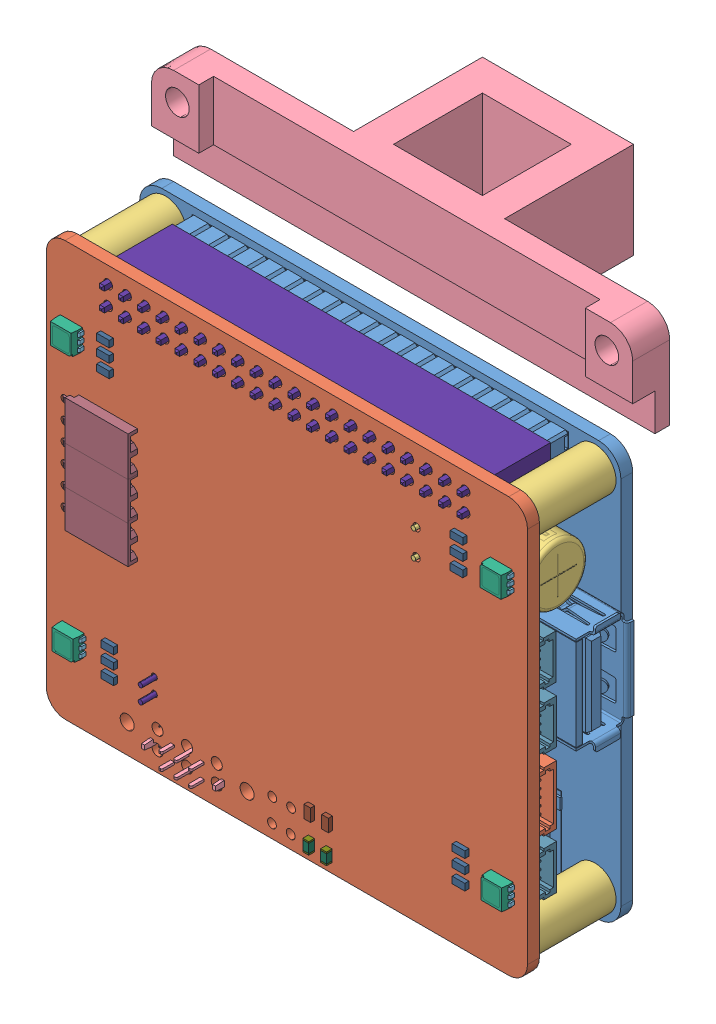
SolidWorks assembly STMf303 hat + RPi 3A+, configuration Default. Lengths in mm.
Overall size (68.17 71.5 38.51).
304 component instances, 41 part files, 9 mates.
Components (placement in the parent):
- Raspberry PI 3 Model A+-1: Raspberry PI 3 Model A+ [Défaut] at (135.3946 10.6154 11.2635) size (68.17 58.5 11.94)
- FC_PiHat_REV1-1: FC_PiHat_REV1 [Default] at (41.2941 -16.4646 23.8635) x (-1 0 0) z (0 0 -1) size (65 56 12.01)
  - FC_PiHat_REV1.step-1: FC_PiHat_REV1.step [Default] at origin size (65 56 12.01)
    - J7FC_PiHat_REV1.step-1: J7FC_PiHat_REV1.step [Default] at origin size (8 4.95 2.96)
      - SM06B-SRSS-TB.step-1: SM06B-SRSS-TB.step [Default] at (13.3 4.6 -0.3) x (1 0 0) z (0 -1 0) size (8 2.96 4.95)
    - C10FC_PiHat_REV1.step-1: C10FC_PiHat_REV1.step [Default] at origin size (13.96 8.06 10.04)
      - User_Library-Cap_electro_8x11_5x3_5mm_RA.step-1: User_Library-Cap_electro_8x11_5x3_5mm_RA.step [Default] at (13.5254 44.5 4) x (0 1 0) z (0 0 1) size (8.06 13.96 10.04)
    - J11FC_PiHat_REV1.step-1: J11FC_PiHat_REV1.step [Default] at origin size (10 6 9.8)
      - User_Library-EG1940-ND.step-1: User_Library-EG1940-ND.step [Default] at (40.9499 0.2249 0) x (1 0 0) z (0 0 1) size (10 6 9.8)
    - D4FC_PiHat_REV1.step-1: D4FC_PiHat_REV1.step [Default] at origin size (3.4 2.8 1.85)
      - User_Library-RGB_LED_Zwart_ASMT-YTC2-0AA02.step-1: User_Library-RGB_LED_Zwart_ASMT-YTC2-0AA02.step [Default] at (2.2908 8.9737 -1.6023) x (-1 0 0) z (0 -1 0) size (3.4 1.85 2.8)
        - Pootje_RGB_LED.step-1: Pootje_RGB_LED.step [Default] at (-0.3594 -0.1975 0.3238) size (0.9 1.1 0.5)
        - ASMT-YTC2-0AA02.step-1: ASMT-YTC2-0AA02.step [Default] at (-2.6594 -0.3475 0.5738) size (3 1.8 2.8)
        - Pootje_RGB_LED.step-2: Pootje_RGB_LED.step [Default] at (-0.3594 -0.1975 -0.5762) size (0.9 1.1 0.5)
        - Pootje_RGB_LED.step-3: Pootje_RGB_LED.step [Default] at (-0.3594 -0.1975 -1.4762) size (0.9 1.1 0.5)
        - Pootje_RGB_LED.step-4: Pootje_RGB_LED.step [Default] at (-1.9594 -0.1975 -1.9762) x (-1 0 0) z (0 0 -1) size (0.9 1.1 0.5)
        - Pootje_RGB_LED.step-5: Pootje_RGB_LED.step [Default] at (-1.9594 -0.1975 -1.0762) x (-1 0 0) z (0 0 -1) size (0.9 1.1 0.5)
        - Pootje_RGB_LED.step-6: Pootje_RGB_LED.step [Default] at (-1.9594 -0.1975 -0.1762) x (-1 0 0) z (0 0 -1) size (0.9 1.1 0.5)
    - D3FC_PiHat_REV1.step-1: D3FC_PiHat_REV1.step [Default] at origin size (3.4 2.8 1.85)
      - User_Library-RGB_LED_Zwart_ASMT-YTC2-0AA02.step-1: User_Library-RGB_LED_Zwart_ASMT-YTC2-0AA02.step [Default] at (2.3908 45.4737 -1.6023) x (-1 0 0) z (0 -1 0) size (3.4 1.85 2.8)
        - Pootje_RGB_LED.step-1: Pootje_RGB_LED.step [Default] at (-0.3594 -0.1975 0.3238) size (0.9 1.1 0.5)
        - ASMT-YTC2-0AA02.step-1: ASMT-YTC2-0AA02.step [Default] at (-2.6594 -0.3475 0.5738) size (3 1.8 2.8)
        - Pootje_RGB_LED.step-2: Pootje_RGB_LED.step [Default] at (-0.3594 -0.1975 -0.5762) size (0.9 1.1 0.5)
        - Pootje_RGB_LED.step-3: Pootje_RGB_LED.step [Default] at (-0.3594 -0.1975 -1.4762) size (0.9 1.1 0.5)
        - Pootje_RGB_LED.step-4: Pootje_RGB_LED.step [Default] at (-1.9594 -0.1975 -1.9762) x (-1 0 0) z (0 0 -1) size (0.9 1.1 0.5)
        - Pootje_RGB_LED.step-5: Pootje_RGB_LED.step [Default] at (-1.9594 -0.1975 -1.0762) x (-1 0 0) z (0 0 -1) size (0.9 1.1 0.5)
        - Pootje_RGB_LED.step-6: Pootje_RGB_LED.step [Default] at (-1.9594 -0.1975 -0.1762) x (-1 0 0) z (0 0 -1) size (0.9 1.1 0.5)
    - D2FC_PiHat_REV1.step-1: D2FC_PiHat_REV1.step [Default] at origin size (3.4 2.8 1.85)
      - User_Library-RGB_LED_Zwart_ASMT-YTC2-0AA02.step-1: User_Library-RGB_LED_Zwart_ASMT-YTC2-0AA02.step [Default] at (62.5092 10.7763 -1.6023) x (1 0 0) z (0 1 0) size (3.4 1.85 2.8)
        - Pootje_RGB_LED.step-1: Pootje_RGB_LED.step [Default] at (-0.3594 -0.1975 0.3238) size (0.9 1.1 0.5)
        - ASMT-YTC2-0AA02.step-1: ASMT-YTC2-0AA02.step [Default] at (-2.6594 -0.3475 0.5738) size (3 1.8 2.8)
        - Pootje_RGB_LED.step-2: Pootje_RGB_LED.step [Default] at (-0.3594 -0.1975 -0.5762) size (0.9 1.1 0.5)
        - Pootje_RGB_LED.step-3: Pootje_RGB_LED.step [Default] at (-0.3594 -0.1975 -1.4762) size (0.9 1.1 0.5)
        - Pootje_RGB_LED.step-4: Pootje_RGB_LED.step [Default] at (-1.9594 -0.1975 -1.9762) x (-1 0 0) z (0 0 -1) size (0.9 1.1 0.5)
        - Pootje_RGB_LED.step-5: Pootje_RGB_LED.step [Default] at (-1.9594 -0.1975 -1.0762) x (-1 0 0) z (0 0 -1) size (0.9 1.1 0.5)
        - Pootje_RGB_LED.step-6: Pootje_RGB_LED.step [Default] at (-1.9594 -0.1975 -0.1762) x (-1 0 0) z (0 0 -1) size (0.9 1.1 0.5)
    - D1FC_PiHat_REV1.step-1: D1FC_PiHat_REV1.step [Default] at origin size (3.4 2.8 1.85)
      - User_Library-RGB_LED_Zwart_ASMT-YTC2-0AA02.step-1: User_Library-RGB_LED_Zwart_ASMT-YTC2-0AA02.step [Default] at (62.7592 46.4263 -1.6023) x (1 0 0) z (0 1 0) size (3.4 1.85 2.8)
        - Pootje_RGB_LED.step-1: Pootje_RGB_LED.step [Default] at (-0.3594 -0.1975 0.3238) size (0.9 1.1 0.5)
        - ASMT-YTC2-0AA02.step-1: ASMT-YTC2-0AA02.step [Default] at (-2.6594 -0.3475 0.5738) size (3 1.8 2.8)
        - Pootje_RGB_LED.step-2: Pootje_RGB_LED.step [Default] at (-0.3594 -0.1975 -0.5762) size (0.9 1.1 0.5)
        - Pootje_RGB_LED.step-3: Pootje_RGB_LED.step [Default] at (-0.3594 -0.1975 -1.4762) size (0.9 1.1 0.5)
        - Pootje_RGB_LED.step-4: Pootje_RGB_LED.step [Default] at (-1.9594 -0.1975 -1.9762) x (-1 0 0) z (0 0 -1) size (0.9 1.1 0.5)
        - Pootje_RGB_LED.step-5: Pootje_RGB_LED.step [Default] at (-1.9594 -0.1975 -1.0762) x (-1 0 0) z (0 0 -1) size (0.9 1.1 0.5)
        - Pootje_RGB_LED.step-6: Pootje_RGB_LED.step [Default] at (-1.9594 -0.1975 -0.1762) x (-1 0 0) z (0 0 -1) size (0.9 1.1 0.5)
    - S1FC_PiHat_REV1.step-1: S1FC_PiHat_REV1.step [Default] at origin size (4.1 4.1 0.81)
      - 5843174976.step-1: 5843174976.step [Default] at (40.7 32.3 0) size (4.1 4.1 0.81)
        - Body.step-1: Body.step [Default] at (-2.05 -2.05 0)
          - Open_CASCADE_STEP_translator_6.8_14.2.1.x_t-1: Open_CASCADE_STEP_translator_6.8_14.2.1.x_t [Default] at origin
        - Open_CASCADE_STEP_translator_6.8_14.1.step-1: Open_CASCADE_STEP_translator_6.8_14.1.step [Default] at (-2.05 -2.05 0) size (0.52 0.52 0.01)
        - Thermal_Shape.step-1: Thermal_Shape.step [Default] at (-1.3 -1.35 -0.001) size (2.6 2.7 0)
        - Pin_Shape.step-1: Pin_Shape.step [Default] at (-2.05 -1.37 0) size (0.35 0.24 0)
        - Pin_Shape.step-2: Pin_Shape.step [Default] at (2.05 1.37 0) x (-1 0 0) z (0 0 1) size (0.35 0.24 0)
        - Pin_Shape.step-3: Pin_Shape.step [Default] at (-2.05 -0.87 0) size (0.35 0.24 0)
        - Pin_Shape.step-4: Pin_Shape.step [Default] at (2.05 0.87 0) x (-1 0 0) z (0 0 1) size (0.35 0.24 0)
        - Pin_Shape.step-5: Pin_Shape.step [Default] at (-2.05 -0.37 0) size (0.35 0.24 0)
        - Pin_Shape.step-6: Pin_Shape.step [Default] at (2.05 0.37 0) x (-1 0 0) z (0 0 1) size (0.35 0.24 0)
        - Pin_Shape.step-7: Pin_Shape.step [Default] at (-2.05 0.13 0) size (0.35 0.24 0)
        - Pin_Shape.step-8: Pin_Shape.step [Default] at (2.05 -0.13 0) x (-1 0 0) z (0 0 1) size (0.35 0.24 0)
        - Pin_Shape.step-9: Pin_Shape.step [Default] at (-2.05 0.63 0) size (0.35 0.24 0)
        - Pin_Shape.step-10: Pin_Shape.step [Default] at (2.05 -0.63 0) x (-1 0 0) z (0 0 1) size (0.35 0.24 0)
        - Pin_Shape.step-11: Pin_Shape.step [Default] at (-2.05 1.13 0) size (0.35 0.24 0)
        - Pin_Shape.step-12: Pin_Shape.step [Default] at (2.05 -1.13 0) x (-1 0 0) z (0 0 1) size (0.35 0.24 0)
        - Pin_Shape.step-13: Pin_Shape.step [Default] at (-1.13 -2.05 0) x (0 1 0) z (0 0 1) size (0.35 0.24 0)
        - Pin_Shape.step-14: Pin_Shape.step [Default] at (1.13 2.05 0) x (0 -1 0) z (0 0 1) size (0.35 0.24 0)
        - Pin_Shape.step-15: Pin_Shape.step [Default] at (-0.63 -2.05 0) x (0 1 0) z (0 0 1) size (0.35 0.24 0)
        - Pin_Shape.step-16: Pin_Shape.step [Default] at (0.63 2.05 0) x (0 -1 0) z (0 0 1) size (0.35 0.24 0)
        - Pin_Shape.step-17: Pin_Shape.step [Default] at (-0.13 -2.05 0) x (0 1 0) z (0 0 1) size (0.35 0.24 0)
        - Pin_Shape.step-18: Pin_Shape.step [Default] at (0.13 2.05 0) x (0 -1 0) z (0 0 1) size (0.35 0.24 0)
        - Pin_Shape.step-19: Pin_Shape.step [Default] at (0.37 -2.05 0) x (0 1 0) z (0 0 1) size (0.35 0.24 0)
        - Pin_Shape.step-20: Pin_Shape.step [Default] at (-0.37 2.05 0) x (0 -1 0) z (0 0 1) size (0.35 0.24 0)
        - Pin_Shape.step-21: Pin_Shape.step [Default] at (0.87 -2.05 0) x (0 1 0) z (0 0 1) size (0.35 0.24 0)
        - Pin_Shape.step-22: Pin_Shape.step [Default] at (-0.87 2.05 0) x (0 -1 0) z (0 0 1) size (0.35 0.24 0)
        - Pin_Shape.step-23: Pin_Shape.step [Default] at (1.37 -2.05 0) x (0 1 0) z (0 0 1) size (0.35 0.24 0)
        - Pin_Shape.step-24: Pin_Shape.step [Default] at (-1.37 2.05 0) x (0 -1 0) z (0 0 1) size (0.35 0.24 0)
    - R14FC_PiHat_REV1.step-1: R14FC_PiHat_REV1.step [Default] at origin size (1.7 0.9 0.55)
      - 6063442624.step-1: 6063442624.step [Default] at (8.7742 7.9 -2.1523) size (1.7 0.9 0.55)
        - Extruded.step-1: Extruded.step [Default] at origin size (1.7 0.9 0.55)
    - R13FC_PiHat_REV1.step-1: R13FC_PiHat_REV1.step [Default] at origin size (1.7 0.9 0.55)
      - 6063442624.step-1: 6063442624.step [Default] at (8.7742 9.8048 -2.1523) size (1.7 0.9 0.55)
        - Extruded.step-1: Extruded.step [Default] at origin size (1.7 0.9 0.55)
    - R12FC_PiHat_REV1.step-1: R12FC_PiHat_REV1.step [Default] at origin size (1.7 0.9 0.55)
      - 6063442624.step-1: 6063442624.step [Default] at (8.7742 11.7 -2.1523) size (1.7 0.9 0.55)
        - Extruded.step-1: Extruded.step [Default] at origin size (1.7 0.9 0.55)
    - R11FC_PiHat_REV1.step-1: R11FC_PiHat_REV1.step [Default] at origin size (1.7 0.9 0.55)
      - 6063442624.step-1: 6063442624.step [Default] at (9.05 44.4 -2.1523) size (1.7 0.9 0.55)
        - Extruded.step-1: Extruded.step [Default] at origin size (1.7 0.9 0.55)
    - R10FC_PiHat_REV1.step-1: R10FC_PiHat_REV1.step [Default] at origin size (1.7 0.9 0.55)
      - 6063442624.step-1: 6063442624.step [Default] at (9.05 46.3 -2.1523) size (1.7 0.9 0.55)
        - Extruded.step-1: Extruded.step [Default] at origin size (1.7 0.9 0.55)
    - R9FC_PiHat_REV1.step-1: R9FC_PiHat_REV1.step [Default] at origin size (0.9 1.7 0.55)
      - 6063442432.step-1: 6063442432.step [Default] at (59.9 29.7 0) size (0.9 1.7 0.55)
        - Extruded-0.step-1: Extruded-0.step [Default] at origin size (0.9 1.7 0.55)
    - R8FC_PiHat_REV1.step-1: R8FC_PiHat_REV1.step [Default] at origin size (1.7 0.9 0.55)
      - 6063442624.step-1: 6063442624.step [Default] at (9.05 48.2 -2.1523) size (1.7 0.9 0.55)
        - Extruded.step-1: Extruded.step [Default] at origin size (1.7 0.9 0.55)
    - R7FC_PiHat_REV1.step-1: R7FC_PiHat_REV1.step [Default] at origin size (1.84 1.84 0.55)
      - 6063441088.step-1: 6063441088.step [Default] at (39.9 37.9 0) size (1.84 1.84 0.55)
        - Extruded-1.step-1: Extruded-1.step [Default] at origin size (1.84 1.84 0.55)
    - R6FC_PiHat_REV1.step-1: R6FC_PiHat_REV1.step [Default] at origin size (1.7 0.9 0.55)
      - 6063442624.step-1: 6063442624.step [Default] at (56.2 11.8 -2.1523) size (1.7 0.9 0.55)
        - Extruded.step-1: Extruded.step [Default] at origin size (1.7 0.9 0.55)
    - R5FC_PiHat_REV1.step-1: R5FC_PiHat_REV1.step [Default] at origin size (1.7 0.9 0.55)
      - 6063442624.step-1: 6063442624.step [Default] at (56.2 10 -2.1523) size (1.7 0.9 0.55)
        - Extruded.step-1: Extruded.step [Default] at origin size (1.7 0.9 0.55)
    - R4FC_PiHat_REV1.step-1: R4FC_PiHat_REV1.step [Default] at origin size (1.7 0.9 0.55)
      - 6063442624.step-1: 6063442624.step [Default] at (56.2 8.2 -2.1523) size (1.7 0.9 0.55)
        - Extruded.step-1: Extruded.step [Default] at origin size (1.7 0.9 0.55)
    - R3FC_PiHat_REV1.step-1: R3FC_PiHat_REV1.step [Default] at origin size (1.7 0.9 0.55)
      - 6063442624.step-1: 6063442624.step [Default] at (56.8 47.4 -2.1523) size (1.7 0.9 0.55)
        - Extruded.step-1: Extruded.step [Default] at origin size (1.7 0.9 0.55)
    - R2FC_PiHat_REV1.step-1: R2FC_PiHat_REV1.step [Default] at origin size (1.7 0.9 0.55)
      - 6063442624.step-1: 6063442624.step [Default] at (56.8 45.6 -2.1523) size (1.7 0.9 0.55)
        - Extruded.step-1: Extruded.step [Default] at origin size (1.7 0.9 0.55)
    - R1FC_PiHat_REV1.step-1: R1FC_PiHat_REV1.step [Default] at origin size (1.7 0.9 0.55)
      - 6063442624.step-1: 6063442624.step [Default] at (56.8 43.8 -2.1523) size (1.7 0.9 0.55)
        - Extruded.step-1: Extruded.step [Default] at origin size (1.7 0.9 0.55)
    - J8FC_PiHat_REV1.step-1: J8FC_PiHat_REV1.step [Default] at origin size (4.95 8 2.96)
      - SM06B-SRSS-TB.step-1: SM06B-SRSS-TB.step [Default] at (4.55 19.8 -0.3) x (0 -1 0) z (-1 0 0) size (8 2.96 4.95)
    - J6FC_PiHat_REV1.step-1: J6FC_PiHat_REV1.step [Default] at origin size (10.06 15.53 5.7)
      - female_header_a-bl254-ea-g02d.step-1: female_header_a-bl254-ea-g02d.step [Default] at (61.2001 31.0851 -1.6023) x (0 -1 0) z (0 0 -1) size (5.33 10.06 5.7)
      - female_header_a-bl254-ea-g02d.step-2: female_header_a-bl254-ea-g02d.step [Default] at (61.2001 26.0099 -1.6023) x (0 -1 0) z (0 0 -1) size (5.33 10.06 5.7)
      - female_header_a-bl254-ea-g02d.step-3: female_header_a-bl254-ea-g02d.step [Default] at (61.2001 36.2099 -1.6023) x (0 -1 0) z (0 0 -1) size (5.33 10.06 5.7)
    - J4FC_PiHat_REV1.step-1: J4FC_PiHat_REV1.step [Default] at origin size (4.95 6 2.96)
      - SM04B-SRSS-TB.step-1: SM04B-SRSS-TB.step [Default] at (4.55 28.375 -0.3) x (0 -1 0) z (-1 0 0) size (6 2.96 4.95)
    - J3FC_PiHat_REV1.step-1: J3FC_PiHat_REV1.step [Default] at origin size (4.95 6 2.96)
      - SM04B-SRSS-TB.step-1: SM04B-SRSS-TB.step [Default] at (4.55 11.35 -0.3) x (0 -1 0) z (-1 0 0) size (6 2.96 4.95)
    - J2FC_PiHat_REV1.step-1: J2FC_PiHat_REV1.step [Default] at origin size (8 4.95 2.96)
      - SM06B-SRSS-TB.step-1: SM06B-SRSS-TB.step [Default] at (22.8093 4.575 -0.3) x (1 0 0) z (0 -1 0) size (8 2.96 4.95)
    - J1FC_PiHat_REV1.step-1: J1FC_PiHat_REV1.step [Default] at origin size (4.95 6 2.96)
      - SM04B-SRSS-TB.step-1: SM04B-SRSS-TB.step [Default] at (4.625 35.925 -0.3) x (0 -1 0) z (-1 0 0) size (6 2.96 4.95)
    - C4FC_PiHat_REV1.step-1: C4FC_PiHat_REV1.step [Default] at origin size (0.9 1.8 0.9)
      - 6063440896.step-1: 6063440896.step [Default] at (41.3 27.825 0) size (0.9 1.8 0.9)
        - Extruded-2.step-1: Extruded-2.step [Default] at origin size (0.9 1.8 0.9)
    - C3FC_PiHat_REV1.step-1: C3FC_PiHat_REV1.step [Default] at origin size (0.9 1.8 0.9)
      - 6063440896.step-1: 6063440896.step [Default] at (44.1 32.225 0) size (0.9 1.8 0.9)
        - Extruded-2.step-1: Extruded-2.step [Default] at origin size (0.9 1.8 0.9)
    - C2FC_PiHat_REV1.step-1: C2FC_PiHat_REV1.step [Default] at origin size (1.8 0.9 0.9)
      - 6063441280.step-1: 6063441280.step [Default] at (38.125 28.8 0) size (1.8 0.9 0.9)
        - Extruded-3.step-1: Extruded-3.step [Default] at origin size (1.8 0.9 0.9)
    - C1FC_PiHat_REV1.step-1: C1FC_PiHat_REV1.step [Default] at origin size (1.8 0.9 0.9)
      - 6063441280.step-1: 6063441280.step [Default] at (38.125 26.7 0) size (1.8 0.9 0.9)
        - Extruded-3.step-1: Extruded-3.step [Default] at origin size (1.8 0.9 0.9)
    - J5FC_PiHat_REV1.step-1: J5FC_PiHat_REV1.step [Default] at origin size (51.1 5 11.1)
      - User_Library-Header_2x20_2_54mm.step-1: User_Library-Header_2x20_2_54mm.step [Default] at (56.6601 52.5601 0) x (1 0 0) z (0 -1 0) size (51.1 11.1 5)
    - L2FC_PiHat_REV1.step-1: L2FC_PiHat_REV1.step [Default] at origin size (12.5 12.7 6.1)
      - 5843174592.step-1: 5843174592.step [Default] at (40.7 17.6 0) x (0 1 0) z (0 0 1) size (12.7 12.5 6.1)
        - pin.step-1: pin.step [Default] at (6.35 2.8 0) x (-1 0 0) z (0 0 1) size (4.5 5.6 3)
          - Open_CASCADE_STEP_translator_6.8_3.3.1.step-1: Open_CASCADE_STEP_translator_6.8_3.3.1.step [Default] at origin size (4.5 5.6 3)
        - pin.step-2: pin.step [Default] at (-6.35 -2.8 0) size (4.5 5.6 3)
          - Open_CASCADE_STEP_translator_6.8_3.3.1.step-1: Open_CASCADE_STEP_translator_6.8_3.3.1.step [Default] at origin size (4.5 5.6 3)
        - Body.step-1: Body.step [Default] at (0 0 0.1)
          - Open_CASCADE_STEP_translator_6.8_14.2.1.x_t-1: Open_CASCADE_STEP_translator_6.8_14.2.1.x_t [Default] at origin
        - cylinder.step-1: cylinder.step [Default] at (0 0 0.1) size (12.5 12.5 3)
    - U3FC_PiHat_REV1.step-1: U3FC_PiHat_REV1.step [Default] at origin size (10.3 15.24 4.47)
      - 5843175168.step-1: 5843175168.step [Default] at (52.775 32.425 0) x (0 1 0) z (0 0 1) size (15.24 10.3 4.47)
        - Body-1.step-1: Body-1.step [Default] at (-4.575 -5.15 0) size (9.15 10.3 4.47)
          - Open_CASCADE_STEP_translator_6.8_42.2.1.step-1: Open_CASCADE_STEP_translator_6.8_42.2.1.step [Default] at origin size (9.15 10.3 4.47)
        - tab.step-1: tab.step [Default] at (-4.575 -5.15 0) size (9 10.25 0.35)
          - Open_CASCADE_STEP_translator_6.8_42.8.1.step-1: Open_CASCADE_STEP_translator_6.8_42.8.1.step [Default] at origin size (9 10.25 0.35)
        - Open_CASCADE_STEP_translator_6.8_42.1.step-1: Open_CASCADE_STEP_translator_6.8_42.1.step [Default] at (-4.575 -5.15 0) size (1.3 1.3 0.01)
        - Lead.step-1: Lead.step [Default] at (-4.575 -3.4 0) x (-1 0 0) z (0 0 1) size (5.46 0.75 2.33)
        - Lead.step-2: Lead.step [Default] at (-4.575 -1.7 0) x (-1 0 0) z (0 0 1) size (5.46 0.75 2.33)
        - Lead.step-3: Lead.step [Default] at (-4.575 0 0) x (-1 0 0) z (0 0 1) size (5.46 0.75 2.33)
        - Lead.step-4: Lead.step [Default] at (-4.575 1.7 0) x (-1 0 0) z (0 0 1) size (5.46 0.75 2.33)
        - Lead.step-5: Lead.step [Default] at (-4.575 3.4 0) x (-1 0 0) z (0 0 1) size (5.46 0.75 2.33)
      - 5843175168-4.step-1: 5843175168-4.step [Default] at (52.775 32.425 0) x (0 1 0) z (0 0 1) size (2.73 0.75 0.2)
    - D6FC_PiHat_REV1.step-1: D6FC_PiHat_REV1.step [Default] at origin size (7.55 6.23 2.62)
      - 5843175552.step-1: 5843175552.step [Default] at (51.8001 16.8001 0) x (1 0 0) z (0 0 1) size (7.55 6.22 2.62)
        - Body-2.step-1: Body-2.step [Default] at (-3.555 -3.11 0.25) size (7.12 6.22 2.47)
          - Open_CASCADE_STEP_translator_6.8_45.1.1.step-1: Open_CASCADE_STEP_translator_6.8_45.1.1.step [Default] at origin size (7.12 6.22 2.47)
        - Lead-5.step-1: Lead-5.step [Default] at (2.635 0 0) size (1.14 3 1.53)
        - Lead-5.step-2: Lead-5.step [Default] at (-2.635 0 0) x (-1 0 0) z (0 0 1) size (1.14 3 1.53)
    - U2FC_PiHat_REV1.step-1: U2FC_PiHat_REV1.step [Default] at origin size (3.98 3.97 1)
      - 5843176128.step-1: 5843176128.step [Default] at (49.3313 45.4354 0) x (0.707107 -0.707107 0) z (0 0 1) size (2.8 2.91 1)
        - Body-3.step-1: Body-3.step [Default] at (-0.8 -1.45 0) size (1.6 2.91 0.95)
          - Open_CASCADE_STEP_translator_6.8_3.1.1.step-1: Open_CASCADE_STEP_translator_6.8_3.1.1.step [Default] at origin size (1.6 2.91 0.95)
        - Leader.step-1: Leader.step [Default] at (-0.8 -0.95 0) x (-1 0 0) z (0 0 1) size (0.6 0.5 0.57)
        - Leader.step-2: Leader.step [Default] at (-0.8 0 0) x (-1 0 0) z (0 0 1) size (0.6 0.5 0.57)
        - Leader.step-3: Leader.step [Default] at (-0.8 0.95 0) x (-1 0 0) z (0 0 1) size (0.6 0.5 0.57)
        - Leader.step-4: Leader.step [Default] at (0.8 -0.95 0) size (0.6 0.5 0.57)
        - Leader.step-5: Leader.step [Default] at (0.8 0.95 0) size (0.6 0.5 0.57)
    - U1FC_PiHat_REV1.step-1: U1FC_PiHat_REV1.step [Default] at origin size (18.98 19.05 1.5)
      - 5843174208.step-1: 5843174208.step [Default] at (26.375 36.65 0) x (-0.707107 -0.707107 0) z (0 0 1) size (14.7 14.7 1.5)
        - Body-4.step-1: Body-4.step [Default] at (-5 -5 0) size (10 10 1.5)
          - Open_CASCADE_STEP_translator_6.8_6.1.1.step-1: Open_CASCADE_STEP_translator_6.8_6.1.1.step [Default] at origin size (10 10 1.5)
        - Leader-6.step-1: Leader-6.step [Default] at (-5 -3.75 0) x (-1 0 0) z (0 0 1) size (2.35 0.27 0.85)
        - Leader-6.step-2: Leader-6.step [Default] at (-3.75 5 0) x (0 1 0) z (0 0 1) size (2.35 0.27 0.85)
        - Leader-6.step-3: Leader-6.step [Default] at (5 -3.75 0) size (2.35 0.27 0.85)
        - Leader-6.step-4: Leader-6.step [Default] at (-3.75 -5 0) x (0 -1 0) z (0 0 1) size (2.35 0.27 0.85)
        - Leader-6.step-5: Leader-6.step [Default] at (-5 -3.25 0) x (-1 0 0) z (0 0 1) size (2.35 0.27 0.85)
        - Leader-6.step-6: Leader-6.step [Default] at (-3.25 5 0) x (0 1 0) z (0 0 1) size (2.35 0.27 0.85)
        - Leader-6.step-7: Leader-6.step [Default] at (5 -3.25 0) size (2.35 0.27 0.85)
        - Leader-6.step-8: Leader-6.step [Default] at (-3.25 -5 0) x (0 -1 0) z (0 0 1) size (2.35 0.27 0.85)
        - Leader-6.step-9: Leader-6.step [Default] at (-5 -2.75 0) x (-1 0 0) z (0 0 1) size (2.35 0.27 0.85)
        - Leader-6.step-10: Leader-6.step [Default] at (-2.75 5 0) x (0 1 0) z (0 0 1) size (2.35 0.27 0.85)
        - Leader-6.step-11: Leader-6.step [Default] at (5 -2.75 0) size (2.35 0.27 0.85)
        - Leader-6.step-12: Leader-6.step [Default] at (-2.75 -5 0) x (0 -1 0) z (0 0 1) size (2.35 0.27 0.85)
        - Leader-6.step-13: Leader-6.step [Default] at (-5 -2.25 0) x (-1 0 0) z (0 0 1) size (2.35 0.27 0.85)
        - Leader-6.step-14: Leader-6.step [Default] at (-2.25 5 0) x (0 1 0) z (0 0 1) size (2.35 0.27 0.85)
        - Leader-6.step-15: Leader-6.step [Default] at (5 -2.25 0) size (2.35 0.27 0.85)
        - Leader-6.step-16: Leader-6.step [Default] at (-2.25 -5 0) x (0 -1 0) z (0 0 1) size (2.35 0.27 0.85)
        - Leader-6.step-17: Leader-6.step [Default] at (-5 -1.75 0) x (-1 0 0) z (0 0 1) size (2.35 0.27 0.85)
        - Leader-6.step-18: Leader-6.step [Default] at (-1.75 5 0) x (0 1 0) z (0 0 1) size (2.35 0.27 0.85)
        - Leader-6.step-19: Leader-6.step [Default] at (5 -1.75 0) size (2.35 0.27 0.85)
        - Leader-6.step-20: Leader-6.step [Default] at (-1.75 -5 0) x (0 -1 0) z (0 0 1) size (2.35 0.27 0.85)
        - Leader-6.step-21: Leader-6.step [Default] at (-5 -1.25 0) x (-1 0 0) z (0 0 1) size (2.35 0.27 0.85)
        - Leader-6.step-22: Leader-6.step [Default] at (-1.25 5 0) x (0 1 0) z (0 0 1) size (2.35 0.27 0.85)
        - Leader-6.step-23: Leader-6.step [Default] at (5 -1.25 0) size (2.35 0.27 0.85)
        - Leader-6.step-24: Leader-6.step [Default] at (-1.25 -5 0) x (0 -1 0) z (0 0 1) size (2.35 0.27 0.85)
        - Leader-6.step-25: Leader-6.step [Default] at (-5 -0.75 0) x (-1 0 0) z (0 0 1) size (2.35 0.27 0.85)
        - Leader-6.step-26: Leader-6.step [Default] at (-0.75 5 0) x (0 1 0) z (0 0 1) size (2.35 0.27 0.85)
        - Leader-6.step-27: Leader-6.step [Default] at (5 -0.75 0) size (2.35 0.27 0.85)
        - Leader-6.step-28: Leader-6.step [Default] at (-0.75 -5 0) x (0 -1 0) z (0 0 1) size (2.35 0.27 0.85)
        - Leader-6.step-29: Leader-6.step [Default] at (-5 -0.25 0) x (-1 0 0) z (0 0 1) size (2.35 0.27 0.85)
        - Leader-6.step-30: Leader-6.step [Default] at (-0.25 5 0) x (0 1 0) z (0 0 1) size (2.35 0.27 0.85)
        - Leader-6.step-31: Leader-6.step [Default] at (5 -0.25 0) size (2.35 0.27 0.85)
        - Leader-6.step-32: Leader-6.step [Default] at (-0.25 -5 0) x (0 -1 0) z (0 0 1) size (2.35 0.27 0.85)
        - Leader-6.step-33: Leader-6.step [Default] at (-5 0.25 0) x (-1 0 0) z (0 0 1) size (2.35 0.27 0.85)
        - Leader-6.step-34: Leader-6.step [Default] at (0.25 5 0) x (0 1 0) z (0 0 1) size (2.35 0.27 0.85)
        - Leader-6.step-35: Leader-6.step [Default] at (5 0.25 0) size (2.35 0.27 0.85)
        - Leader-6.step-36: Leader-6.step [Default] at (0.25 -5 0) x (0 -1 0) z (0 0 1) size (2.35 0.27 0.85)
        - Leader-6.step-37: Leader-6.step [Default] at (-5 0.75 0) x (-1 0 0) z (0 0 1) size (2.35 0.27 0.85)
        - Leader-6.step-38: Leader-6.step [Default] at (0.75 5 0) x (0 1 0) z (0 0 1) size (2.35 0.27 0.85)
        - Leader-6.step-39: Leader-6.step [Default] at (5 0.75 0) size (2.35 0.27 0.85)
        - Leader-6.step-40: Leader-6.step [Default] at (0.75 -5 0) x (0 -1 0) z (0 0 1) size (2.35 0.27 0.85)
        - Leader-6.step-41: Leader-6.step [Default] at (-5 1.25 0) x (-1 0 0) z (0 0 1) size (2.35 0.27 0.85)
        - Leader-6.step-42: Leader-6.step [Default] at (1.25 5 0) x (0 1 0) z (0 0 1) size (2.35 0.27 0.85)
        - Leader-6.step-43: Leader-6.step [Default] at (5 1.25 0) size (2.35 0.27 0.85)
        - Leader-6.step-44: Leader-6.step [Default] at (1.25 -5 0) x (0 -1 0) z (0 0 1) size (2.35 0.27 0.85)
        - Leader-6.step-45: Leader-6.step [Default] at (-5 1.75 0) x (-1 0 0) z (0 0 1) size (2.35 0.27 0.85)
        - Leader-6.step-46: Leader-6.step [Default] at (1.75 5 0) x (0 1 0) z (0 0 1) size (2.35 0.27 0.85)
        - Leader-6.step-47: Leader-6.step [Default] at (5 1.75 0) size (2.35 0.27 0.85)
        - Leader-6.step-48: Leader-6.step [Default] at (1.75 -5 0) x (0 -1 0) z (0 0 1) size (2.35 0.27 0.85)
        - Leader-6.step-49: Leader-6.step [Default] at (-5 2.25 0) x (-1 0 0) z (0 0 1) size (2.35 0.27 0.85)
        - Leader-6.step-50: Leader-6.step [Default] at (2.25 5 0) x (0 1 0) z (0 0 1) size (2.35 0.27 0.85)
        - Leader-6.step-51: Leader-6.step [Default] at (5 2.25 0) size (2.35 0.27 0.85)
        - Leader-6.step-52: Leader-6.step [Default] at (2.25 -5 0) x (0 -1 0) z (0 0 1) size (2.35 0.27 0.85)
        - Leader-6.step-53: Leader-6.step [Default] at (-5 2.75 0) x (-1 0 0) z (0 0 1) size (2.35 0.27 0.85)
        - Leader-6.step-54: Leader-6.step [Default] at (2.75 5 0) x (0 1 0) z (0 0 1) size (2.35 0.27 0.85)
        - Leader-6.step-55: Leader-6.step [Default] at (5 2.75 0) size (2.35 0.27 0.85)
        - Leader-6.step-56: Leader-6.step [Default] at (2.75 -5 0) x (0 -1 0) z (0 0 1) size (2.35 0.27 0.85)
        - Leader-6.step-57: Leader-6.step [Default] at (-5 3.25 0) x (-1 0 0) z (0 0 1) size (2.35 0.27 0.85)
        - Leader-6.step-58: Leader-6.step [Default] at (3.25 5 0) x (0 1 0) z (0 0 1) size (2.35 0.27 0.85)
        - Leader-6.step-59: Leader-6.step [Default] at (5 3.25 0) size (2.35 0.27 0.85)
        - Leader-6.step-60: Leader-6.step [Default] at (3.25 -5 0) x (0 -1 0) z (0 0 1) size (2.35 0.27 0.85)
        - Leader-6.step-61: Leader-6.step [Default] at (-5 3.75 0) x (-1 0 0) z (0 0 1) size (2.35 0.27 0.85)
        - Leader-6.step-62: Leader-6.step [Default] at (3.75 5 0) x (0 1 0) z (0 0 1) size (2.35 0.27 0.85)
        - Leader-6.step-63: Leader-6.step [Default] at (5 3.75 0) size (2.35 0.27 0.85)
        - Leader-6.step-64: Leader-6.step [Default] at (3.75 -5 0) x (0 -1 0) z (0 0 1) size (2.35 0.27 0.85)
    - R17FC_PiHat_REV1.step-1: R17FC_PiHat_REV1.step [Default] at origin size (0.9 1.7 0.55)
      - 6063442432.step-1: 6063442432.step [Default] at (29.2 5.9 -2.1523) size (0.9 1.7 0.55)
        - Extruded-0.step-1: Extruded-0.step [Default] at origin size (0.9 1.7 0.55)
    - R15FC_PiHat_REV1.step-1: R15FC_PiHat_REV1.step [Default] at origin size (0.9 1.7 0.55)
      - 6063442432.step-1: 6063442432.step [Default] at (26.8 5.9 -2.1523) size (0.9 1.7 0.55)
        - Extruded-0.step-1: Extruded-0.step [Default] at origin size (0.9 1.7 0.55)
    - Q1FC_PiHat_REV1.step-1: Q1FC_PiHat_REV1.step [Default] at origin size (3.2 5 1.35)
      - User_Library-445-CRYTAL-SMD.step-1: User_Library-445-CRYTAL-SMD.step [Default] at (37.4671 49.9363 0.0126) x (0 1 0) z (1 0 0) size (5 1.35 3.2)
    - L3FC_PiHat_REV1.step-1: L3FC_PiHat_REV1.step [Default] at origin size (12.5 12.7 6.1)
      - 5843174592.step-1: 5843174592.step [Default] at (27.5 17.6 0) x (0 1 0) z (0 0 1) size (12.7 12.5 6.1)
        - pin.step-1: pin.step [Default] at (6.35 2.8 0) x (-1 0 0) z (0 0 1) size (4.5 5.6 3)
          - Open_CASCADE_STEP_translator_6.8_3.3.1.step-1: Open_CASCADE_STEP_translator_6.8_3.3.1.step [Default] at origin size (4.5 5.6 3)
        - pin.step-2: pin.step [Default] at (-6.35 -2.8 0) size (4.5 5.6 3)
          - Open_CASCADE_STEP_translator_6.8_3.3.1.step-1: Open_CASCADE_STEP_translator_6.8_3.3.1.step [Default] at origin size (4.5 5.6 3)
        - Body.step-1: Body.step [Default] at (0 0 0.1)
          - Open_CASCADE_STEP_translator_6.8_14.2.1.x_t-1: Open_CASCADE_STEP_translator_6.8_14.2.1.x_t [Default] at origin
        - cylinder.step-1: cylinder.step [Default] at (0 0 0.1) size (12.5 12.5 3)
    - L1FC_PiHat_REV1.step-1: L1FC_PiHat_REV1.step [Default] at origin size (3.68 3.68 1.5)
      - 6063441856.step-1: 6063441856.step [Default] at (51.5 42 0) size (3.68 3.68 1.5)
        - Extruded-7.step-1: Extruded-7.step [Default] at origin size (3.68 3.68 1.5)
    - D7FC_PiHat_REV1.step-1: D7FC_PiHat_REV1.step [Default] at origin size (0.8 1.6 0.75)
      - 6063441664.step-1: 6063441664.step [Default] at (29.2 2.1 -2.3523) size (0.8 1.2 0.75)
        - Extruded-8.step-1: Extruded-8.step [Default] at origin size (0.8 1.2 0.75)
      - 6063441472.step-1: 6063441472.step [Default] at (29.2 2.8 -2.3523) size (0.8 0.2 0.75)
        - Extruded-9.step-1: Extruded-9.step [Default] at origin size (0.8 0.2 0.75)
      - 6063441472.step-2: 6063441472.step [Default] at (29.2 1.4 -2.3523) size (0.8 0.2 0.75)
        - Extruded-9.step-1: Extruded-9.step [Default] at origin size (0.8 0.2 0.75)
    - D5FC_PiHat_REV1.step-1: D5FC_PiHat_REV1.step [Default] at origin size (0.8 1.6 0.75)
      - 6063441664.step-1: 6063441664.step [Default] at (26.8 2.075 -2.3523) size (0.8 1.2 0.75)
        - Extruded-8.step-1: Extruded-8.step [Default] at origin size (0.8 1.2 0.75)
      - 6063441472.step-1: 6063441472.step [Default] at (26.8 2.775 -2.3523) size (0.8 0.2 0.75)
        - Extruded-9.step-1: Extruded-9.step [Default] at origin size (0.8 0.2 0.75)
      - 6063441472.step-2: 6063441472.step [Default] at (26.8 1.375 -2.3523) size (0.8 0.2 0.75)
        - Extruded-9.step-1: Extruded-9.step [Default] at origin size (0.8 0.2 0.75)
    - C9FC_PiHat_REV1.step-1: C9FC_PiHat_REV1.step [Default] at origin size (13.46 5.06 8.54)
      - User_Library-Cap_electro_5x11x2mm_RA.step-1: User_Library-Cap_electro_5x11x2mm_RA.step [Default] at (51.885 9.9755 2.5) x (0 -1 0) z (0 0 1) size (5.06 13.46 8.54)
    - C8FC_PiHat_REV1.step-1: C8FC_PiHat_REV1.step [Default] at origin size (1.91 1.91 0.9)
      - 6063442048.step-1: 6063442048.step [Default] at (47.1 43.3857 0) size (1.91 1.91 0.9)
        - Extruded-10.step-1: Extruded-10.step [Default] at origin size (1.91 1.91 0.9)
    - C7FC_PiHat_REV1.step-1: C7FC_PiHat_REV1.step [Default] at origin size (1.91 1.91 0.9)
      - 6063442240.step-1: 6063442240.step [Default] at (45.7 46.4 0) size (1.91 1.91 0.9)
        - Extruded-11.step-1: Extruded-11.step [Default] at origin size (1.91 1.91 0.9)
    - C6FC_PiHat_REV1.step-1: C6FC_PiHat_REV1.step [Default] at origin size (1.8 0.9 0.9)
      - 6063441280.step-1: 6063441280.step [Default] at (39.9535 42.2416 0) size (1.8 0.9 0.9)
        - Extruded-3.step-1: Extruded-3.step [Default] at origin size (1.8 0.9 0.9)
    - C5FC_PiHat_REV1.step-1: C5FC_PiHat_REV1.step [Default] at origin size (1.8 0.9 0.9)
      - 6063441280.step-1: 6063441280.step [Default] at (39.9535 44.9915 0) size (1.8 0.9 0.9)
        - Extruded-3.step-1: Extruded-3.step [Default] at origin size (1.8 0.9 0.9)
    - BoardFC_PiHat_REV1.step-1: BoardFC_PiHat_REV1.step [Default] at origin size (65 56 1.6)
- Spacer-1: Spacer [Default] at (37.7941 -12.9363 12.8635) x (-1 0 0) z (0 1 0) size (5.7 11 5.7)
- Spacer-2: Spacer [Default] at (-20.2059 -12.9363 12.8635) x (1 0 0) z (0 -1 0) size (5.7 11 5.7)
- Spacer-3: Spacer [Default] at (-20.2059 36.0637 12.8635) x (1 0 0) z (0 -1 0) size (5.7 11 5.7)
- Spacer-4: Spacer [Default] at (37.7941 36.0637 12.8635) x (-1 0 0) z (0 1 0) size (5.7 11 5.7)
- Part1^STMf303 hat + RPi 3A+-1: Part1^STMf303 hat + RPi 3A+ [Default] at (41.2941 -16.4646 25.4659) x (1 0 0) z (0 0 1) size (65 13 22.4) (virtual)
Mates (geometry in assembly coordinates):
- Coincident1: coincident anti-aligned: plane of Raspberry PI 3 Model A+-1 through (-15.4142 35.0854 15.3635) normal (0 0 1); plane of FC_PiHat_REV1-1/FC_PiHat_REV1.step-1/J5FC_PiHat_REV1.step-1/User_Library-Header_2x20_2_54mm.step-1 through (-13.946 33.5954 15.3635) normal (0 0 -1)
- Coincident2: coincident aligned: plane of Raspberry PI 3 Model A+-1 through (-23.7059 11.5637 12.8635) normal (-1 0 0); plane of FC_PiHat_REV1-1/FC_PiHat_REV1.step-1/BoardFC_PiHat_REV1.step-1 through (-23.7059 36.9954 25.4659) normal (-1 0 0)
- Coincident10: coincident: plane of Raspberry PI 3 Model A+-1 through (33.8158 38.5954 12.8635) normal (0 1 0); line of FC_PiHat_REV1-1/FC_PiHat_REV1.step-1/J5FC_PiHat_REV1.step-1/User_Library-Header_2x20_2_54mm.step-1 through (34.314 38.5954 23.8635) axis (0 0 -1)
- Coincident11: coincident anti-aligned: plane of Raspberry PI 3 Model A+-1 through (18.7941 11.5637 12.8635) normal (0 0 1); plane of Spacer-1 through (37.7941 -12.9363 12.8635) normal (0 0 -1)
- Concentric1: concentric anti-aligned: cylinder of Raspberry PI 3 Model A+-1 through (37.7941 -12.9363 12.8635) axis (0 0 -1) radius 1.375; circle of Spacer-1
- InPlace1: in place: plane of FC_PiHat_REV1-1/FC_PiHat_REV1.step-1/BoardFC_PiHat_REV1.step-1 through (-21.1659 39.5354 25.4659) normal (0 0 1); plane of ? through (0 0 25.4659) normal (0 0 1); moOrthogonalPlaneRef_w of FC_PiHat_REV1-1/FC_PiHat_REV1.step-1/BoardFC_PiHat_REV1.step-1 through (-21.1659 39.5354 25.4659) normal (0 0 1); plane of ? through (0 0 25.4659) normal (0 1 0); plane of FC_PiHat_REV1-1/FC_PiHat_REV1.step-1/BoardFC_PiHat_REV1.step-1 through (-21.1659 39.5354 25.4659) normal (0 0 1); plane of ? through (0 0 25.4659) normal (1 0 0); plane of FC_PiHat_REV1-1/FC_PiHat_REV1.step-1/BoardFC_PiHat_REV1.step-1 through (-21.1659 39.5354 25.4659) normal (0 0 1); unknown of Part1^STMf303 hat + RPi 3A+-1
- Coincident12: coincident aligned: plane of FC_PiHat_REV1-1/FC_PiHat_REV1.step-1/BoardFC_PiHat_REV1.step-1; plane of Part1^STMf303 hat + RPi 3A+-1
- Coincident13: coincident aligned: moOrthogonalPlaneRef_w of FC_PiHat_REV1-1/FC_PiHat_REV1.step-1/BoardFC_PiHat_REV1.step-1 through (41.2941 -16.4646 25.4659) normal (0 1 0); plane of Part1^STMf303 hat + RPi 3A+-1 through (41.2941 -16.4646 25.4659) normal (0 1 0)
- Coincident14: coincident anti-aligned: moOrthogonalPlaneRef_w of FC_PiHat_REV1-1/FC_PiHat_REV1.step-1/BoardFC_PiHat_REV1.step-1 through (41.2941 -16.4646 25.4659) normal (-1 0 0); plane of Part1^STMf303 hat + RPi 3A+-1 through (41.2941 -16.4646 25.4659) normal (1 0 0)
